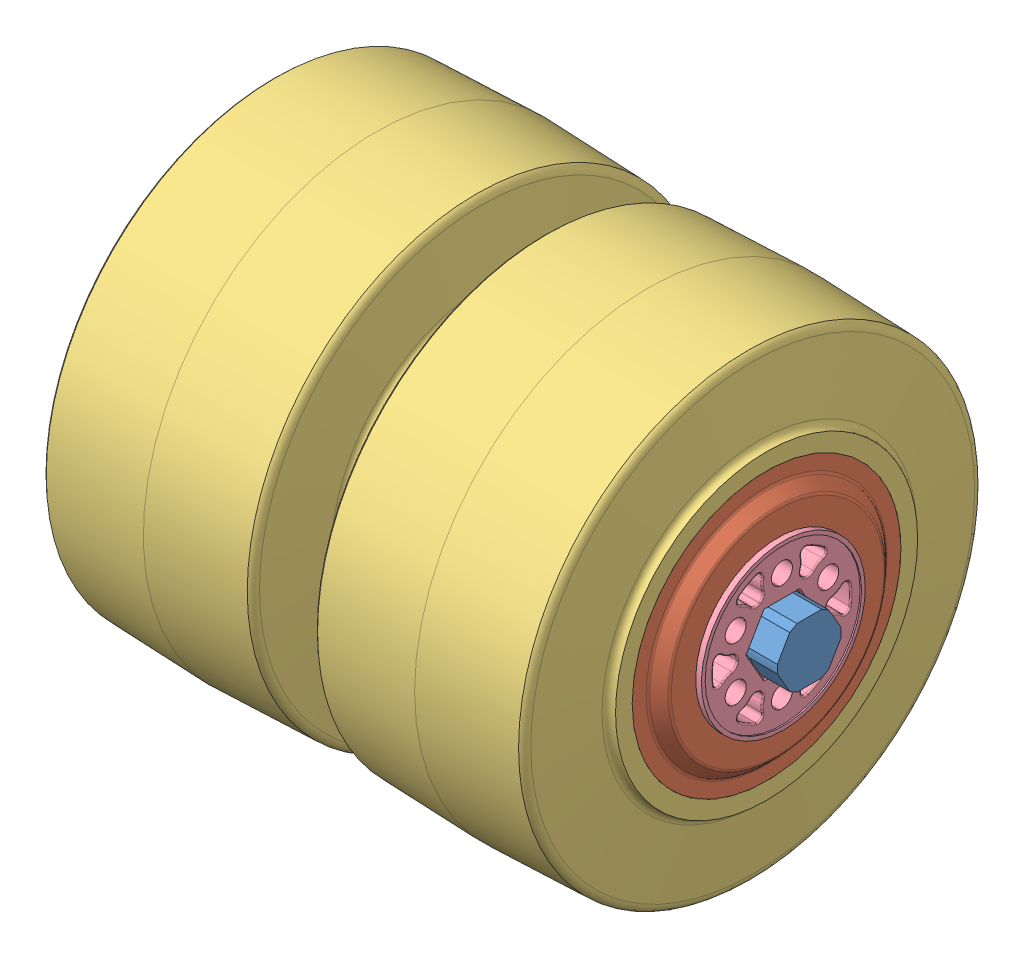
SolidWorks assembly flywheel_assembly - GreyT Shooter (Falcon VP Direct), configuration Default. Lengths in mm.
Overall size (127 136.01 136.01).
10 component instances, 4 part files, 7 mates.
Components (placement in the parent):
- flywheel_bar - GreyT Shooter (Falcon VP Direct)-1: flywheel_bar - GreyT Shooter (Falcon VP Direct) [Default] at (0 14.5144 16.3745) size (127 12.7 13.75)
  - WCP-0281-007 Rev1-1: WCP-0281-007 Rev1 [Default] at origin size (127 12.7 13.75)
- 2in_flywheel_w_hex (217-4054)-1: 2in_flywheel_w_hex (217-4054) [Default] at (-28.9766 14.5144 16.3598) x (1 0 0) z (0 0.866025 0.5) size (57.95 99.57 99.57)
  - 217-4054-003 Rev1-1: 217-4054-003 Rev1 [Default] at origin size (55.55 82.55 82.55)
  - 217-4054-004 Rev1-1: 217-4054-004 Rev1 [Default] at origin size (50.8 99.57 99.57)
  - 217-4054-002 Rev15-1: 217-4054-002 Rev15 [Default] x (0 0 1) z (-1 0 0) size (50.79 50.79 57.95)
- 2in_flywheel_w_hex (217-4054)-2: 2in_flywheel_w_hex (217-4054) [Default] at (28.9766 14.5398 16.3745) size (57.95 99.57 99.57)
  - 217-4054-003 Rev1-1: 217-4054-003 Rev1 [Default] at origin size (55.55 82.55 82.55)
  - 217-4054-004 Rev1-1: 217-4054-004 Rev1 [Default] at origin size (50.8 99.57 99.57)
  - 217-4054-002 Rev15-1: 217-4054-002 Rev15 [Default] x (0 0 1) z (-1 0 0) size (50.79 50.79 57.95)
Mates (geometry in assembly coordinates):
- Coincident2: coincident aligned: plane of flywheel_bar - GreyT Shooter (Falcon VP Direct)-1/WCP-0281-007 Rev1-1 through (0 14.5144 16.3745) normal (1 0 0)
- Coincident5: coincident anti-aligned: plane of flywheel_bar - GreyT Shooter (Falcon VP Direct)-1/WCP-0281-007 Rev1-1 through (57.15 11.3394 21.8737) normal (0 -0.5 0.866025); plane of 2in_flywheel_w_hex (217-4054)-1/217-4054-002 Rev15-1 through (-57.6532 8.1517 20.0333) normal (0 0.5 -0.866025)
- Coincident6: coincident anti-aligned: plane of flywheel_bar - GreyT Shooter (Falcon VP Direct)-1/WCP-0281-007 Rev1-1 through (57.15 11.3394 21.8737) normal (0 -0.5 0.866025); plane of 2in_flywheel_w_hex (217-4054)-2/217-4054-002 Rev15-1 through (0.3 8.1771 20.048) normal (0 0.5 -0.866025)
- Coincident7: coincident anti-aligned: plane of flywheel_bar - GreyT Shooter (Falcon VP Direct)-1/WCP-0281-007 Rev1-1 through (57.15 11.3394 10.8752) normal (0 -0.5 -0.866025); plane of 2in_flywheel_w_hex (217-4054)-2/217-4054-002 Rev15-1 through (0.3 14.5398 9.0275) normal (0 0.5 0.866025)
- Coincident8: coincident anti-aligned: plane of flywheel_bar - GreyT Shooter (Falcon VP Direct)-1/WCP-0281-007 Rev1-1 through (57.15 17.6894 21.8737) normal (0 0.5 0.866025); plane of 2in_flywheel_w_hex (217-4054)-1/217-4054-002 Rev15-1 through (-57.6532 14.5144 23.7068) normal (0 -0.5 -0.866025)
- Coincident13: coincident aligned: plane of 2in_flywheel_w_hex (217-4054)-1/217-4054-002 Rev15-1 through (0 14.5144 16.3598) normal (1 0 0)
- Coincident14: coincident anti-aligned: plane of 2in_flywheel_w_hex (217-4054)-2/217-4054-002 Rev15-1 through (0 14.5398 16.3745) normal (-1 0 0)
